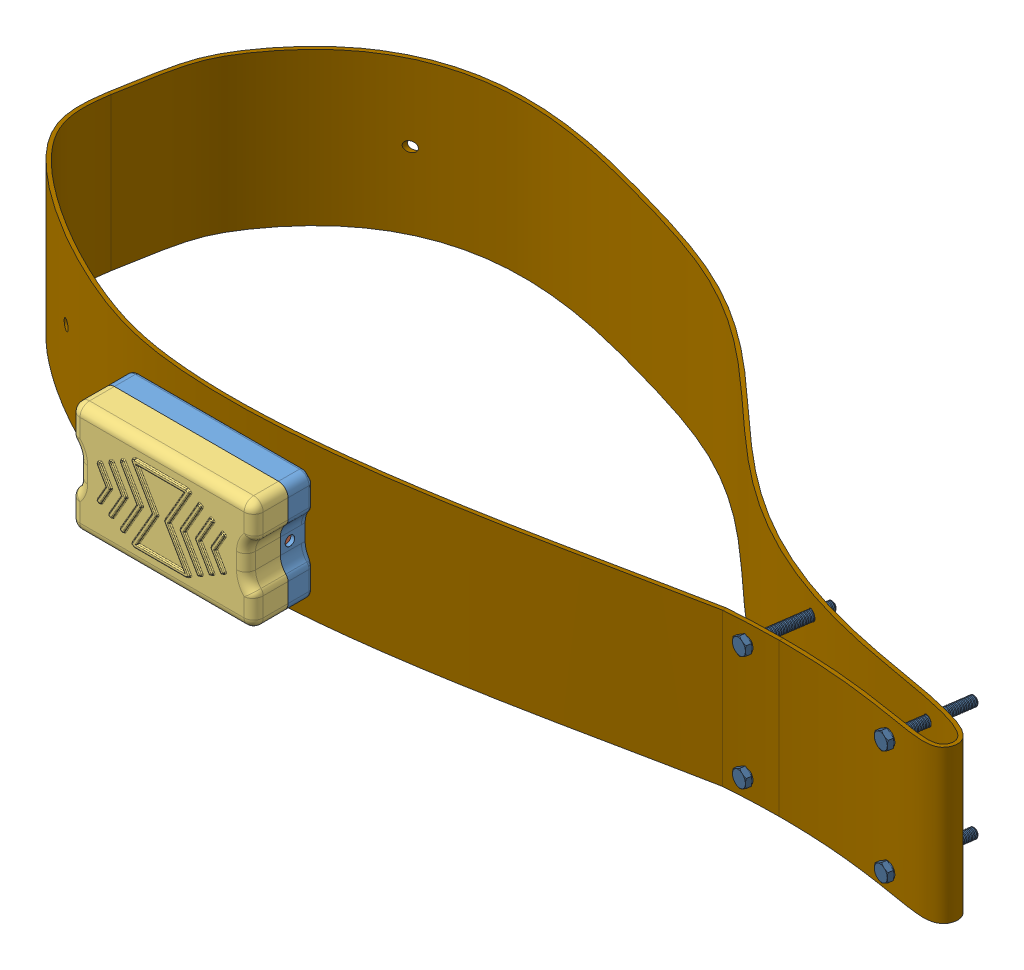
SolidWorks assembly СБ Корпус Peggy Tracker, configuration По умолчанию. Lengths in mm.
Overall size (548.26 80.13 407.1).
306 component instances, 82 part files, 15 mates.
Components (placement in the parent):
- Case-01-1: Case-01 [По умолчанию] at (217.6814 215.7743 273.7334) size (339.05 58 369.63)
- Аккумулятор литий-полимерный LP115181-1: Аккумулятор литий-полимерный LP115181 [Default] at (177.1814 219.2743 275.7334) size (81 51 11)
- Case-02-1: Case-02 [По умолчанию] at (217.6814 215.7743 304.7334) x (-1 0 0) z (0 0 -1) size (96 58 19)
- Печатная плата Peggy Tracker-1: Печатная плата Peggy Tracker [По умолчанию] at (183.6814 227.2743 296.1739) x (0 1 0) z (0 0 -1) size (35 62 10.1)
  - Печатная плата Peggy Tracker.step-1: Печатная плата Peggy Tracker.step [Default] at origin size (35 62 10.1)
    - Board.step-1: Board.step [Default] at origin size (35 62 1.56)
      - Open CASCADE STEP translator 6.8 1.1.1.step-1: Open CASCADE STEP translator 6.8 1.1.1.step [Default] at (0 0 -1.5596) size (35 62 1.56)
    - X1.step-1: X1.step [Default] at origin size (28 20 6.7)
      - 6517451856.step-1: 6517451856.step [Default] at (11.15 51.75 6) size (3 3 0.7)
        - Extruded.step-1: Extruded.step [Default] at origin size (3 3 0.7)
      - 6517450176.step-1: 6517450176.step [Default] at (9.1815 45.8445 6) size (6.22 4.19 0.7)
        - Extruded-0.step-1: Extruded-0.step [Default] at origin size (6.22 4.19 0.7)
      - 6517450176.step-2: 6517450176.step [Default] at (9.1815 57.6545 6) size (6.22 4.19 0.7)
        - Extruded-0.step-1: Extruded-0.step [Default] at origin size (6.22 4.19 0.7)
      - 6517449536.step-1: 6517449536.step [Default] at (4.785 51.7495 0) size (2.57 16 6.7)
        - Extruded-1.step-1: Extruded-1.step [Default] at origin size (2.57 16 6.7)
      - 6517449376.step-1: 6517449376.step [Default] at (8.1819 51.7635 6) size (4.22 2.41 0.7)
        - Extruded-2.step-1: Extruded-2.step [Default] at origin size (4.22 2.41 0.7)
      - 6517449056.step-1: 6517449056.step [Default] at (30.8492 51.7495 0) size (1.3 16 6.7)
        - Extruded-3.step-1: Extruded-3.step [Default] at origin size (1.3 16 6.7)
      - 6517448576.step-1: 6517448576.step [Default] at (28.9305 45.5257 6) size (2.54 3.55 0.7)
        - Extruded-4.step-1: Extruded-4.step [Default] at origin size (2.54 3.55 0.7)
      - 6517448256.step-1: 6517448256.step [Default] at (29.4382 51.4325 6) size (1.52 5.71 0.7)
        - Extruded-5.step-1: Extruded-5.step [Default] at origin size (1.52 5.71 0.7)
      - 6517447856.step-1: 6517447856.step [Default] at (18.1354 51.7495 0) size (24.13 16 1)
        - Extruded-6.step-1: Extruded-6.step [Default] at origin size (24.13 16 1)
      - 6517447456.step-1: 6517447456.step [Default] at (18.135 58.925 0) size (24.13 1.65 2.5)
        - Extruded-7.step-1: Extruded-7.step [Default] at origin size (24.13 1.65 2.5)
      - 6517447456.step-2: 6517447456.step [Default] at (18.1356 44.5737 0) size (24.13 1.65 2.5)
        - Extruded-7.step-1: Extruded-7.step [Default] at origin size (24.13 1.65 2.5)
      - 6517447056.step-1: 6517447056.step [Default] at (19.0875 48.7663 0) size (9.53 0.89 2.5)
        - Extruded-8.step-1: Extruded-8.step [Default] at origin size (9.53 0.89 2.5)
      - 6517447056.step-2: 6517447056.step [Default] at (19.0875 54.2273 0) size (9.53 0.89 2.5)
        - Extruded-8.step-1: Extruded-8.step [Default] at origin size (9.53 0.89 2.5)
      - 6517446256.step-1: 6517446256.step [Default] at (28.9302 57.972 6) size (2.54 3.55 0.7)
        - Extruded-9.step-1: Extruded-9.step [Default] at origin size (2.54 3.55 0.7)
      - CircuitWorks-BATT_CR2032.step-1: CircuitWorks-BATT_CR2032.step [Default] at (17.5 51.75 6) x (1 0 0) z (0 1 0) size (20 3.2 20)
    - XW2.step-1: XW2.step [Default] at origin size (2.86 3.01 1.29)
      - IPX.step-1: IPX.step [Default] at (2.0669 38.1281 1.27) x (0 1 0) z (0 0 1) size (3.01 2.86 1.29)
    - XW1.step-1: XW1.step [Default] at origin size (2.86 3.01 1.29)
      - IPX.step-1: IPX.step [Default] at (1.9653 7.4677 1.27) x (0 1 0) z (0 0 1) size (3.01 2.86 1.29)
    - R6.step-1: R6.step [Default] at origin size (0.9 1.7 0.55)
      - 6482559680.step-1: 6482559680.step [Default] at (28.8001 34.2999 0) x (0 -1 0) z (0 0 1) size (1.7 0.9 0.55)
        - Terminal.step-1: Terminal.step [Default] at (-0.85 -0.45 0) size (0.1 0.9 0.55)
          - Open_CASCADE_STEP_translator_6.8_15.2.1.step-1: Open_CASCADE_STEP_translator_6.8_15.2.1.step [Default] at origin size (0.1 0.9 0.55)
        - Terminal.step-2: Terminal.step [Default] at (0.85 0.45 0) x (-1 0 0) z (0 0 1) size (0.1 0.9 0.55)
          - Open_CASCADE_STEP_translator_6.8_15.2.1.step-1: Open_CASCADE_STEP_translator_6.8_15.2.1.step [Default] at origin size (0.1 0.9 0.55)
        - Mid_Body.step-1: Mid_Body.step [Default] at (-0.85 -0.45 0) size (1.59 0.9 0.44)
        - Mark.step-1: Mark.step [Default] at (-0.75 -0.45 0.495) size (1.5 0.9 0.06)
    - X3.step-1: X3.step [Default] at origin size (4.5 5.9 9.4)
      - B2B-PH-K-S(LF)(SN)--3DModel-STEP-56544.step-1: B2B-PH-K-S(LF)(SN)--3DModel-STEP-56544.step [Default] at (32.5449 33.0001 3) x (0 -1 0) z (-1 0 0) size (5.9 9.4 4.5)
    - R5.step-1: R5.step [Default] at origin size (0.95 1.75 0.95)
      - 6482560720.step-1: 6482560720.step [Default] at (27.1578 23.3326 0) x (0 1 0) z (0 0 1) size (1.75 0.95 0.95)
        - Terminal-1.step-1: Terminal-1.step [Default] at (-0.875 -0.475 0) size (0.2 0.95 0.95)
          - Open_CASCADE_STEP_translator_6.8_12.2.1.step-1: Open_CASCADE_STEP_translator_6.8_12.2.1.step [Default] at origin size (0.2 0.95 0.95)
        - Terminal-1.step-2: Terminal-1.step [Default] at (0.875 0.475 0) x (-1 0 0) z (0 0 1) size (0.2 0.95 0.95)
          - Open_CASCADE_STEP_translator_6.8_12.2.1.step-1: Open_CASCADE_STEP_translator_6.8_12.2.1.step [Default] at origin size (0.2 0.95 0.95)
        - Mid_Body-10.step-1: Mid_Body-10.step [Default] at (-0.875 -0.475 0) size (1.56 0.95 0.76)
        - Mark-11.step-1: Mark-11.step [Default] at (-0.675 -0.475 0.855) size (1.35 0.95 0.1)
    - R4.step-1: R4.step [Default] at origin size (0.95 1.75 0.95)
      - 6482560720.step-1: 6482560720.step [Default] at (27.1578 25.8726 0) x (0 1 0) z (0 0 1) size (1.75 0.95 0.95)
        - Terminal-1.step-1: Terminal-1.step [Default] at (-0.875 -0.475 0) size (0.2 0.95 0.95)
          - Open_CASCADE_STEP_translator_6.8_12.2.1.step-1: Open_CASCADE_STEP_translator_6.8_12.2.1.step [Default] at origin size (0.2 0.95 0.95)
        - Terminal-1.step-2: Terminal-1.step [Default] at (0.875 0.475 0) x (-1 0 0) z (0 0 1) size (0.2 0.95 0.95)
          - Open_CASCADE_STEP_translator_6.8_12.2.1.step-1: Open_CASCADE_STEP_translator_6.8_12.2.1.step [Default] at origin size (0.2 0.95 0.95)
        - Mid_Body-10.step-1: Mid_Body-10.step [Default] at (-0.875 -0.475 0) size (1.56 0.95 0.76)
        - Mark-11.step-1: Mark-11.step [Default] at (-0.675 -0.475 0.855) size (1.35 0.95 0.1)
    - R3.step-1: R3.step [Default] at origin size (0.9 1.7 0.55)
      - 6482559680.step-1: 6482559680.step [Default] at (28.8001 31.7999 0) x (0 -1 0) z (0 0 1) size (1.7 0.9 0.55)
        - Terminal.step-1: Terminal.step [Default] at (-0.85 -0.45 0) size (0.1 0.9 0.55)
          - Open_CASCADE_STEP_translator_6.8_15.2.1.step-1: Open_CASCADE_STEP_translator_6.8_15.2.1.step [Default] at origin size (0.1 0.9 0.55)
        - Terminal.step-2: Terminal.step [Default] at (0.85 0.45 0) x (-1 0 0) z (0 0 1) size (0.1 0.9 0.55)
          - Open_CASCADE_STEP_translator_6.8_15.2.1.step-1: Open_CASCADE_STEP_translator_6.8_15.2.1.step [Default] at origin size (0.1 0.9 0.55)
        - Mid_Body.step-1: Mid_Body.step [Default] at (-0.85 -0.45 0) size (1.59 0.9 0.44)
        - Mark.step-1: Mark.step [Default] at (-0.75 -0.45 0.495) size (1.5 0.9 0.06)
    - R2.step-1: R2.step [Default] at origin size (0.9 1.7 0.55)
      - 6482559840.step-1: 6482559840.step [Default] at (24.5109 16.5497 0) x (0 1 0) z (0 0 1) size (1.7 0.9 0.55)
        - Terminal-2.step-1: Terminal-2.step [Default] at (-0.85 -0.45 0) size (0.1 0.9 0.55)
          - Open_CASCADE_STEP_translator_6.8_15.2.1-12.step-1: Open_CASCADE_STEP_translator_6.8_15.2.1-12.step [Default] at origin size (0.1 0.9 0.55)
        - Terminal-2.step-2: Terminal-2.step [Default] at (0.85 0.45 0) x (-1 0 0) z (0 0 1) size (0.1 0.9 0.55)
          - Open_CASCADE_STEP_translator_6.8_15.2.1-12.step-1: Open_CASCADE_STEP_translator_6.8_15.2.1-12.step [Default] at origin size (0.1 0.9 0.55)
        - Mid_Body-13.step-1: Mid_Body-13.step [Default] at (-0.85 -0.45 0) size (1.59 0.9 0.44)
        - Mark-14.step-1: Mark-14.step [Default] at (-0.75 -0.45 0.495) size (1.5 0.9 0.06)
    - R1.step-1: R1.step [Default] at origin size (1.7 0.9 0.55)
      - 6517452256.step-1: 6517452256.step [Default] at (8.2043 34.8489 0) size (1.7 0.9 0.55)
        - Terminal-3.step-1: Terminal-3.step [Default] at (-0.85 -0.45 0) size (0.1 0.9 0.55)
          - Open_CASCADE_STEP_translator_6.8_15.2.1-15.step-1: Open_CASCADE_STEP_translator_6.8_15.2.1-15.step [Default] at origin size (0.1 0.9 0.55)
        - Terminal-3.step-2: Terminal-3.step [Default] at (0.85 0.45 0) x (-1 0 0) z (0 0 1) size (0.1 0.9 0.55)
          - Open_CASCADE_STEP_translator_6.8_15.2.1-15.step-1: Open_CASCADE_STEP_translator_6.8_15.2.1-15.step [Default] at origin size (0.1 0.9 0.55)
        - Mid_Body-16.step-1: Mid_Body-16.step [Default] at (-0.85 -0.45 0) size (1.59 0.9 0.44)
        - Mark-17.step-1: Mark-17.step [Default] at (-0.75 -0.45 0.495) size (1.5 0.9 0.06)
    - L2.step-1: L2.step [Default] at origin size (5.2 5.2 1.8)
      - 6482573440.step-1: 6482573440.step [Default] at (30.1268 13.8076 0.2) x (1 0 0) z (0 -1 0) size (5.2 1.8 5.2)
    - L1.step-1: L1.step [Default] at origin size (0.95 1.75 0.95)
      - 6482561680.step-1: 6482561680.step [Default] at (5.85 37.366 0) x (0 1 0) z (0 0 1) size (1.75 0.95 0.95)
        - Terminal-4.step-1: Terminal-4.step [Default] at (-0.875 -0.475 0) size (1.75 0.95 0.95)
          - Open_CASCADE_STEP_translator_6.8_2.1.1.step-1: Open_CASCADE_STEP_translator_6.8_2.1.1.step [Default] at origin size (0.2 0.95 0.95)
          - Open_CASCADE_STEP_translator_6.8_2.1.2.step-1: Open_CASCADE_STEP_translator_6.8_2.1.2.step [Default] at origin size (0.2 0.95 0.95)
        - Mid_Body-18.step-1: Mid_Body-18.step [Default] at (-0.875 -0.475 0) size (1.35 0.95 0.95)
          - Open_CASCADE_STEP_translator_6.8_2.2.1.step-1: Open_CASCADE_STEP_translator_6.8_2.2.1.step [Default] at origin size (1.35 0.95 0.95)
    - DD2.step-1: DD2.step [Default] at origin size (15 15.5 3.52)
      - 3D_RAK3172.step-1: 3D_RAK3172.step [Default] at (20.536 20.4601 1) x (-1 0 0) z (0 0 1) size (15 15.5 3.52)
        - Board-1.step-1: Board-1.step [Default] at origin size (15 15.5 1.01)
          - Open_CASCADE_STEP_translator_6.8_1.1.1.step-1: Open_CASCADE_STEP_translator_6.8_1.1.1.step [Default] at (0 0 -1.014) size (15 15.5 1.01)
            - Open_CASCADE_STEP_translator_6.8_1.1.1.1.step-1: Open_CASCADE_STEP_translator_6.8_1.1.1.1.step [Default] at origin size (15 15.5 1.01)
        - R11.step-1: R11.step [Default] at origin size (0.6 0.3 0.3)
          - 0201_SMD_Capacitor.step-1: 0201_SMD_Capacitor.step [Default] at (3.4751 6.9342 0.2794) x (-1 0 0) z (0 0 1) size (0.6 0.3 0.3)
        - U2.step-1: U2.step [Default] at origin size (0.99 1.02 0.75)
          - 6590464912.step-1: 6590464912.step [Default] at (5.4483 13.05 0) size (0.99 1.02 0.75)
            - Extruded-19.step-1: Extruded-19.step [Default] at origin size (0.99 1.02 0.75)
        - R4-1.step-1: R4-1.step [Default] at origin size (0.68 0.33 0.34)
          - R0201.step-1: R0201.step [Default] at (3.9176 5.9192 0) x (1 0 0) z (0 -1 0) size (0.68 0.34 0.33)
        - R3-1.step-1: R3-1.step [Default] at origin size (0.33 0.68 0.34)
          - R0201.step-1: R0201.step [Default] at (4.1676 5.6692 0) x (0 1 0) z (1 0 0) size (0.68 0.34 0.33)
        - L2-1.step-1: L2-1.step [Default] at origin size (1.15 0.55 0.41)
          - RES_1005-0402.step-1: RES_1005-0402.step [Default] at (2.2661 6.0198 0) x (1 0 0) z (0 -1 0) size (1.15 0.41 0.55)
        - C10.step-1: C10.step [Default] at origin size (0.6 0.3 0.3)
          - 0201_SMD_Capacitor.step-1: 0201_SMD_Capacitor.step [Default] at (7.1835 13.462 0.2794) x (-1 0 0) z (0 0 1) size (0.6 0.3 0.3)
        - C9.step-1: C9.step [Default] at origin size (0.6 0.3 0.3)
          - 0201_SMD_Capacitor.step-1: 0201_SMD_Capacitor.step [Default] at (7.1835 13.97 0.2794) x (-1 0 0) z (0 0 1) size (0.6 0.3 0.3)
        - C8.step-1: C8.step [Default] at origin size (0.6 0.3 0.3)
          - 0201_SMD_Capacitor.step-1: 0201_SMD_Capacitor.step [Default] at (7.1835 12.954 0.2794) x (-1 0 0) z (0 0 1) size (0.6 0.3 0.3)
        - C7.step-1: C7.step [Default] at origin size (0.6 0.3 0.3)
          - 0201_SMD_Capacitor.step-1: 0201_SMD_Capacitor.step [Default] at (6.0793 11.938 0.2794) x (1 0 0) z (0 0 1) size (0.6 0.3 0.3)
        - C6.step-1: C6.step [Default] at origin size (0.6 0.3 0.3)
          - 0201_SMD_Capacitor.step-1: 0201_SMD_Capacitor.step [Default] at (3.8855 13.5541 0.2794) x (-1 0 0) z (0 0 1) size (0.6 0.3 0.3)
        - CON1.step-1: CON1.step [Default] at origin size (3.4 3.1 1.25)
          - UFL-R-SMD.step-1: UFL-R-SMD.step [Default] at (11.3537 12.7757 0) x (1 0 0) z (0 0 1) size (3.4 3.1 1.25)
            - Part_525.step-1: Part_525.step [Default] at origin size (3 2.6 0.35)
            - Part_739.step-1: Part_739.step [Default] at origin size (2 2 0.9)
            - Part_578.step-1: Part_578.step [Default] at origin size (0.6 0.5 0.1)
            - Part_540.step-1: Part_540.step [Default] at origin size (0.4 1.8 0.1)
            - Part_562.step-1: Part_562.step [Default] at origin size (0.4 1.8 0.1)
            - Part_555.step-1: Part_555.step [Default] at origin size (0.6 0.5 0.1)
        - C4.step-1: C4.step [Default] at origin size (0.6 0.3 0.3)
          - 0201_SMD_Capacitor.step-1: 0201_SMD_Capacitor.step [Default] at (3.7799 9.398 0.2794) x (-1 0 0) z (0 0 1) size (0.6 0.3 0.3)
        - U1.step-1: U1.step [Default] at origin size (7.02 7.02 0.8)
          - QFN48_7x7.step-1: QFN48_7x7.step [Default] at (8.8366 6.9818 0) x (0 1 0) z (1 0 0) size (7.02 0.8 7.02)
        - X1-1.step-1: X1-1.step [Default] at origin size (1.61 2.01 0.71)
          - NT2016SA.step-1: NT2016SA.step [Default] at (1.7496 8.4946 0) x (0 1 0) z (1 0 0) size (2.01 0.71 1.61)
        - C43.step-1: C43.step [Default] at origin size (0.6 0.3 0.3)
          - 0201_SMD_Capacitor.step-1: 0201_SMD_Capacitor.step [Default] at (3.7799 9.9822 0.2794) x (-1 0 0) z (0 0 1) size (0.6 0.3 0.3)
        - C42.step-1: C42.step [Default] at origin size (0.3 0.6 0.3)
          - 0201_SMD_Capacitor.step-1: 0201_SMD_Capacitor.step [Default] at (3.0734 7.9709 0.2794) x (0 -1 0) z (0 0 1) size (0.6 0.3 0.3)
        - R9.step-1: R9.step [Default] at origin size (0.6 0.3 0.3)
          - 0201_SMD_Capacitor.step-1: 0201_SMD_Capacitor.step [Default] at (3.7799 8.8138 0.2794) x (-1 0 0) z (0 0 1) size (0.6 0.3 0.3)
        - C1.step-1: C1.step [Default] at origin size (0.6 0.3 0.3)
          - 0201_SMD_Capacitor.step-1: 0201_SMD_Capacitor.step [Default] at (7.0445 11.557 0.2794) x (1 0 0) z (0 0 1) size (0.6 0.3 0.3)
        - C2.step-1: C2.step [Default] at origin size (0.3 0.6 0.3)
          - 0201_SMD_Capacitor.step-1: 0201_SMD_Capacitor.step [Default] at (7.9756 12.2635 0.2794) x (0 -1 0) z (0 0 1) size (0.6 0.3 0.3)
        - C3.step-1: C3.step [Default] at origin size (0.3 0.6 0.3)
          - 0201_SMD_Capacitor.step-1: 0201_SMD_Capacitor.step [Default] at (2.1844 13.4518 0.2794) x (0 -1 0) z (0 0 1) size (0.6 0.3 0.3)
        - C11.step-1: C11.step [Default] at origin size (0.6 0.3 0.3)
          - 0201_SMD_Capacitor.step-1: 0201_SMD_Capacitor.step [Default] at (1.6623 11.9866 0.2794) x (1 0 0) z (0 0 1) size (0.6 0.3 0.3)
        - C12.step-1: C12.step [Default] at origin size (0.6 0.3 0.3)
          - 0201_SMD_Capacitor.step-1: 0201_SMD_Capacitor.step [Default] at (3.2813 12.573 0.2794) x (1 0 0) z (0 0 1) size (0.6 0.3 0.3)
        - C13.step-1: C13.step [Default] at origin size (0.3 0.6 0.3)
          - 0201_SMD_Capacitor.step-1: 0201_SMD_Capacitor.step [Default] at (4.4958 12.0697 0.2794) x (0 1 0) z (0 0 1) size (0.6 0.3 0.3)
        - C14.step-1: C14.step [Default] at origin size (0.3 0.6 0.3)
          - 0201_SMD_Capacitor.step-1: 0201_SMD_Capacitor.step [Default] at (2.7178 12.6739 0.2794) x (0 -1 0) z (0 0 1) size (0.6 0.3 0.3)
        - C17.step-1: C17.step [Default] at origin size (0.3 0.6 0.3)
          - 0201_SMD_Capacitor.step-1: 0201_SMD_Capacitor.step [Default] at (7.6708 14.4693 0.2794) x (0 -1 0) z (0 0 1) size (0.6 0.3 0.3)
        - C18.step-1: C18.step [Default] at origin size (0.6 0.3 0.3)
          - 0201_SMD_Capacitor.step-1: 0201_SMD_Capacitor.step [Default] at (9.1901 14.1224 0.2794) x (-1 0 0) z (0 0 1) size (0.6 0.3 0.3)
        - C19.step-1: C19.step [Default] at origin size (0.3 0.6 0.3)
          - 0201_SMD_Capacitor.step-1: 0201_SMD_Capacitor.step [Default] at (2.8814 10.8799 0.2794) x (0 1 0) z (0 0 1) size (0.6 0.3 0.3)
        - C22.step-1: C22.step [Default] at origin size (0.3 0.6 0.3)
          - 0201_SMD_Capacitor.step-1: 0201_SMD_Capacitor.step [Default] at (2.0432 11.4801 0.2794) x (0 -1 0) z (0 0 1) size (0.6 0.3 0.3)
        - C21.step-1: C21.step [Default] at origin size (0.3 0.6 0.3)
          - 0201_SMD_Capacitor.step-1: 0201_SMD_Capacitor.step [Default] at (1.5606 11.4801 0.2794) x (0 -1 0) z (0 0 1) size (0.6 0.3 0.3)
        - C23.step-1: C23.step [Default] at origin size (1 0.5 0.5)
          - C0402.step-1: C0402.step [Default] at (8.9644 1.5539 0.254) x (1 0 0) z (0 0 1) size (1 0.5 0.5)
        - C24.step-1: C24.step [Default] at origin size (0.6 0.3 0.3)
          - 0201_SMD_Capacitor.step-1: 0201_SMD_Capacitor.step [Default] at (4.7197 3.8862 0.2794) x (-1 0 0) z (0 0 1) size (0.6 0.3 0.3)
        - C26.step-1: C26.step [Default] at origin size (0.3 0.6 0.3)
          - 0201_SMD_Capacitor.step-1: 0201_SMD_Capacitor.step [Default] at (10.541 2.2265 0.2794) x (0 -1 0) z (0 0 1) size (0.6 0.3 0.3)
        - C44.step-1: C44.step [Default] at origin size (0.6 0.3 0.3)
          - 0201_SMD_Capacitor.step-1: 0201_SMD_Capacitor.step [Default] at (4.7919 9.9822 0.2794) x (-1 0 0) z (0 0 1) size (0.6 0.3 0.3)
        - C29.step-1: C29.step [Default] at origin size (0.6 0.3 0.3)
          - 0201_SMD_Capacitor.step-1: 0201_SMD_Capacitor.step [Default] at (3.9925 7.8486 0.2794) x (1 0 0) z (0 0 1) size (0.6 0.3 0.3)
        - C25.step-1: C25.step [Default] at origin size (0.3 0.6 0.3)
          - 0201_SMD_Capacitor.step-1: 0201_SMD_Capacitor.step [Default] at (10.287 1.6263 0.2794) x (0 1 0) z (0 0 1) size (0.6 0.3 0.3)
        - C31.step-1: C31.step [Default] at origin size (0.6 0.3 0.3)
          - 0201_SMD_Capacitor.step-1: 0201_SMD_Capacitor.step [Default] at (3.9965 7.239 0.2794) x (1 0 0) z (0 0 1) size (0.6 0.3 0.3)
        - C32.step-1: C32.step [Default] at origin size (0.6 0.3 0.3)
          - 0201_SMD_Capacitor.step-1: 0201_SMD_Capacitor.step [Default] at (7.8533 2.3622 0.2794) x (1 0 0) z (0 0 1) size (0.6 0.3 0.3)
        - C33.step-1: C33.step [Default] at origin size (1 0.5 0.5)
          - C0402.step-1: C0402.step [Default] at (5.3048 2.0461 0.254) x (-1 0 0) z (0 0 1) size (1 0.5 0.5)
        - C34.step-1: C34.step [Default] at origin size (0.3 0.6 0.3)
          - 0201_SMD_Capacitor.step-1: 0201_SMD_Capacitor.step [Default] at (4.318 4.2211 0.2794) x (0 1 0) z (0 0 1) size (0.6 0.3 0.3)
        - C35.step-1: C35.step [Default] at origin size (0.6 0.3 0.3)
          - 0201_SMD_Capacitor.step-1: 0201_SMD_Capacitor.step [Default] at (9.0365 2.3622 0.2794) x (1 0 0) z (0 0 1) size (0.6 0.3 0.3)
        - C36.step-1: C36.step [Default] at origin size (0.3 0.6 0.3)
          - 0201_SMD_Capacitor.step-1: 0201_SMD_Capacitor.step [Default] at (13.0302 10.0751 0.2794) x (0 -1 0) z (0 0 1) size (0.6 0.3 0.3)
        - C37.step-1: C37.step [Default] at origin size (0.3 0.6 0.3)
          - 0201_SMD_Capacitor.step-1: 0201_SMD_Capacitor.step [Default] at (3.7338 4.2211 0.2794) x (0 1 0) z (0 0 1) size (0.6 0.3 0.3)
        - C38.step-1: C38.step [Default] at origin size (1 0.5 0.5)
          - C0402.step-1: C0402.step [Default] at (2.3114 4.7323 0.254) x (1 0 0) z (0 0 1) size (1 0.5 0.5)
        - C39.step-1: C39.step [Default] at origin size (0.6 0.3 0.3)
          - 0201_SMD_Capacitor.step-1: 0201_SMD_Capacitor.step [Default] at (4.0593 3.1881 0.2794) x (-1 0 0) z (0 0 1) size (0.6 0.3 0.3)
        - C40.step-1: C40.step [Default] at origin size (0.3 0.6 0.3)
          - 0201_SMD_Capacitor.step-1: 0201_SMD_Capacitor.step [Default] at (3.6576 1.7319 0.2794) x (0 1 0) z (0 0 1) size (0.6 0.3 0.3)
        - L1-1.step-1: L1-1.step [Default] at origin size (0.68 0.33 0.34)
          - R0201.step-1: R0201.step [Default] at (7.8526 11.2014 0) x (-1 0 0) z (0 1 0) size (0.68 0.34 0.33)
        - L3.step-1: L3.step [Default] at origin size (0.33 0.68 0.34)
          - R0201.step-1: R0201.step [Default] at (1.7272 13.1318 0) x (0 -1 0) z (-1 0 0) size (0.68 0.34 0.33)
        - L5.step-1: L5.step [Default] at origin size (0.68 0.33 0.34)
          - R0201.step-1: R0201.step [Default] at (8.0772 13.3096 0) x (-1 0 0) z (0 1 0) size (0.68 0.34 0.33)
        - L6.step-1: L6.step [Default] at origin size (1 0.5 0.5)
          - C0402.step-1: C0402.step [Default] at (5.822 11.0823 0.254) x (1 0 0) z (0 0 1) size (1 0.5 0.5)
        - L7.step-1: L7.step [Default] at origin size (0.68 0.33 0.34)
          - R0201.step-1: R0201.step [Default] at (3.5854 12.1158 0) x (1 0 0) z (0 -1 0) size (0.68 0.34 0.33)
        - L9.step-1: L9.step [Default] at origin size (1.15 0.55 0.41)
          - RES_1005-0402.step-1: RES_1005-0402.step [Default] at (3.9641 11.3538 0) x (-1 0 0) z (0 1 0) size (1.15 0.41 0.55)
        - L20.step-1: L20.step [Default] at origin size (1.6 0.8 0.3)
          - 6559637360.step-1: 6559637360.step [Default] at (12.3698 2.0828 0) x (-1 0 0) z (0 1 0) size (1.6 0.3 0.8)
        - L30.step-1: L30.step [Default] at origin size (1.15 0.55 0.41)
          - RES_1005-0402.step-1: RES_1005-0402.step [Default] at (7.1263 1.8 0) x (-1 0 0) z (0 1 0) size (1.15 0.41 0.55)
        - X2.step-1: X2.step [Default] at origin size (1.2 2 0.61)
          - crystal_rtf2012.step-1: crystal_rtf2012.step [Default] at (2.25 2.8402 0) x (0 1 0) z (1 0 0) size (2 0.61 1.2)
        - R2-1.step-1: R2-1.step [Default] at origin size (0.68 0.33 0.34)
          - R0201.step-1: R0201.step [Default] at (1.9613 10.1854 0) x (1 0 0) z (0 -1 0) size (0.68 0.34 0.33)
        - C5.step-1: C5.step [Default] at origin size (0.6 0.3 0.3)
          - 0201_SMD_Capacitor.step-1: 0201_SMD_Capacitor.step [Default] at (1.8749 6.9342 0.2794) x (-1 0 0) z (0 0 1) size (0.6 0.3 0.3)
        - Free-Models.step-1: Free-Models.step [Default] at origin size (13.4 13.9 2.5)
          - D030A-______.step-1: D030A-______.step [Default] at (2.429 -1.8288 0) size (13.4 13.9 2.5)
    - DD1.step-1: DD1.step [Default] at origin size (9.7 10.1 2.8)
      - 6482566000.step-1: 6482566000.step [Default] at (16.1 34.85 0) x (1 0 0) z (0 0 1) size (9.7 10.1 2.8)
        - Body.step-1: Body.step [Default] at (0 0 0.1) size (9.7 10.1 2.7)
        - Pins.step-1: Pins.step [Default] at origin size (9.56 9.36 0.1)
    - DA1.step-1: DA1.step [Default] at origin size (3 3 1)
      - 6482561360.step-1: 6482561360.step [Default] at (31.2728 20.6686 0) x (0 1 0) z (0 0 1) size (3 3 1)
        - FRAME-DRC0010J.step-1: FRAME-DRC0010J.step [Default] x (1 0 0) z (0 -1 0) size (3 0.2 3)
          - Open CASCADE STEP translator 6.8 1.16.1.2.1.step-1: Open CASCADE STEP translator 6.8 1.16.1.2.1.step [Default] at origin size (1.9 0.2 3)
          - Open CASCADE STEP translator 6.8 1.16.1.2.2.step-1: Open CASCADE STEP translator 6.8 1.16.1.2.2.step [Default] at origin size (0.4 0.2 0.24)
          - Open CASCADE STEP translator 6.8 1.16.1.2.3.step-1: Open CASCADE STEP translator 6.8 1.16.1.2.3.step [Default] at origin size (0.4 0.2 0.24)
          - Open CASCADE STEP translator 6.8 1.16.1.2.4.step-1: Open CASCADE STEP translator 6.8 1.16.1.2.4.step [Default] at origin size (0.4 0.2 0.24)
          - Open CASCADE STEP translator 6.8 1.16.1.2.5.step-1: Open CASCADE STEP translator 6.8 1.16.1.2.5.step [Default] at origin size (0.4 0.2 0.24)
          - Open CASCADE STEP translator 6.8 1.16.1.2.6.step-1: Open CASCADE STEP translator 6.8 1.16.1.2.6.step [Default] at origin size (0.4 0.2 0.24)
          - Open CASCADE STEP translator 6.8 1.16.1.2.7.step-1: Open CASCADE STEP translator 6.8 1.16.1.2.7.step [Default] at origin size (0.4 0.2 0.24)
          - Open CASCADE STEP translator 6.8 1.16.1.2.8.step-1: Open CASCADE STEP translator 6.8 1.16.1.2.8.step [Default] at origin size (0.4 0.2 0.24)
          - Open CASCADE STEP translator 6.8 1.16.1.2.9.step-1: Open CASCADE STEP translator 6.8 1.16.1.2.9.step [Default] at origin size (0.4 0.2 0.24)
          - Open CASCADE STEP translator 6.8 1.16.1.2.10.step-1: Open CASCADE STEP translator 6.8 1.16.1.2.10.step [Default] at origin size (0.4 0.2 0.24)
          - Open CASCADE STEP translator 6.8 1.16.1.2.11.step-1: Open CASCADE STEP translator 6.8 1.16.1.2.11.step [Default] at origin size (0.4 0.2 0.24)
        - BODY-SON.step-1: BODY-SON.step [Default] at (0 0 0.025) x (1 0 0) z (0 -1 0) size (3 0.97 3)
    - C8-1.step-1: C8-1.step [Default] at origin size (1.4 2.15 1.4)
      - 6482573680.step-1: 6482573680.step [Default] at (27.1929 19.9035 0) x (0 -1 0) z (0 0 1) size (2.15 1.4 1.4)
        - Terminal-5.step-1: Terminal-5.step [Default] at (-1.075 -0.7 0) size (2.15 1.4 1.4)
          - Open_CASCADE_STEP_translator_6.8_5.1.1.step-1: Open_CASCADE_STEP_translator_6.8_5.1.1.step [Default] at origin size (0.2 1.4 1.4)
          - Open_CASCADE_STEP_translator_6.8_5.1.2.step-1: Open_CASCADE_STEP_translator_6.8_5.1.2.step [Default] at origin size (0.2 1.4 1.4)
        - Mid_Body-1.step-1: Mid_Body-1.step [Default] at (-1.075 -0.7 0) size (1.75 1.4 1.4)
          - Open_CASCADE_STEP_translator_6.8_5.2.1.step-1: Open_CASCADE_STEP_translator_6.8_5.2.1.step [Default] at origin size (1.75 1.4 1.4)
    - C7-1.step-1: C7-1.step [Default] at origin size (2.1 1.35 1.35)
      - 6482573600.step-1: 6482573600.step [Default] at (31.889 26.8 0) x (1 0 0) z (0 0 1) size (2.1 1.35 1.35)
        - Terminal-6.step-1: Terminal-6.step [Default] at (-1.05 -0.675 0) size (2.1 1.35 1.35)
          - Open_CASCADE_STEP_translator_6.8_24.1.1.step-1: Open_CASCADE_STEP_translator_6.8_24.1.1.step [Default] at origin size (0.2 1.35 1.35)
          - Open_CASCADE_STEP_translator_6.8_24.1.2.step-1: Open_CASCADE_STEP_translator_6.8_24.1.2.step [Default] at origin size (0.2 1.35 1.35)
        - Mid_Body-2.step-1: Mid_Body-2.step [Default] at (-1.05 -0.675 0) size (1.7 1.35 1.35)
          - Open_CASCADE_STEP_translator_6.8_24.2.1.step-1: Open_CASCADE_STEP_translator_6.8_24.2.1.step [Default] at origin size (1.7 1.35 1.35)
    - C6-1.step-1: C6-1.step [Default] at origin size (0.9 1.7 0.9)
      - 6482559520.step-1: 6482559520.step [Default] at (22.727 16.763 0) x (0 -1 0) z (0 0 1) size (1.7 0.9 0.9)
        - Terminal-7.step-1: Terminal-7.step [Default] at (-0.85 -0.45 0) size (1.7 0.9 0.9)
          - Open_CASCADE_STEP_translator_6.8_5.1.1-20.step-1: Open_CASCADE_STEP_translator_6.8_5.1.1-20.step [Default] at origin size (0.2 0.9 0.9)
          - Open_CASCADE_STEP_translator_6.8_5.1.2-21.step-1: Open_CASCADE_STEP_translator_6.8_5.1.2-21.step [Default] at origin size (0.2 0.9 0.9)
        - Mid_Body-3.step-1: Mid_Body-3.step [Default] at (-0.85 -0.45 0) size (1.3 0.9 0.9)
          - Open_CASCADE_STEP_translator_6.8_5.2.1-22.step-1: Open_CASCADE_STEP_translator_6.8_5.2.1-22.step [Default] at origin size (1.3 0.9 0.9)
    - C5-1.step-1: C5-1.step [Default] at origin size (1.35 2.1 1.35)
      - 6482568960.step-1: 6482568960.step [Default] at (24.505 19.939 0) x (0 -1 0) z (0 0 1) size (2.1 1.35 1.35)
        - Terminal-8.step-1: Terminal-8.step [Default] at (-1.05 -0.675 0) size (2.1 1.35 1.35)
          - Open_CASCADE_STEP_translator_6.8_24.1.1-23.step-1: Open_CASCADE_STEP_translator_6.8_24.1.1-23.step [Default] at origin size (0.2 1.35 1.35)
          - Open_CASCADE_STEP_translator_6.8_24.1.2-24.step-1: Open_CASCADE_STEP_translator_6.8_24.1.2-24.step [Default] at origin size (0.2 1.35 1.35)
        - Mid_Body-4.step-1: Mid_Body-4.step [Default] at (-1.05 -0.675 0) size (1.7 1.35 1.35)
          - Open_CASCADE_STEP_translator_6.8_24.2.1-25.step-1: Open_CASCADE_STEP_translator_6.8_24.2.1-25.step [Default] at origin size (1.7 1.35 1.35)
    - C4-1.step-1: C4-1.step [Default] at origin size (0.9 1.7 0.9)
      - 6482559520.step-1: 6482559520.step [Default] at (22.7 19.888 0) x (0 -1 0) z (0 0 1) size (1.7 0.9 0.9)
        - Terminal-7.step-1: Terminal-7.step [Default] at (-0.85 -0.45 0) size (1.7 0.9 0.9)
          - Open_CASCADE_STEP_translator_6.8_5.1.1-20.step-1: Open_CASCADE_STEP_translator_6.8_5.1.1-20.step [Default] at origin size (0.2 0.9 0.9)
          - Open_CASCADE_STEP_translator_6.8_5.1.2-21.step-1: Open_CASCADE_STEP_translator_6.8_5.1.2-21.step [Default] at origin size (0.2 0.9 0.9)
        - Mid_Body-3.step-1: Mid_Body-3.step [Default] at (-0.85 -0.45 0) size (1.3 0.9 0.9)
          - Open_CASCADE_STEP_translator_6.8_5.2.1-22.step-1: Open_CASCADE_STEP_translator_6.8_5.2.1-22.step [Default] at origin size (1.3 0.9 0.9)
    - C3-1.step-1: C3-1.step [Default] at origin size (1.35 2.1 1.35)
      - 6482568960.step-1: 6482568960.step [Default] at (25.7048 39.0008 0) x (0 -1 0) z (0 0 1) size (2.1 1.35 1.35)
        - Terminal-8.step-1: Terminal-8.step [Default] at (-1.05 -0.675 0) size (2.1 1.35 1.35)
          - Open_CASCADE_STEP_translator_6.8_24.1.1-23.step-1: Open_CASCADE_STEP_translator_6.8_24.1.1-23.step [Default] at origin size (0.2 1.35 1.35)
          - Open_CASCADE_STEP_translator_6.8_24.1.2-24.step-1: Open_CASCADE_STEP_translator_6.8_24.1.2-24.step [Default] at origin size (0.2 1.35 1.35)
        - Mid_Body-4.step-1: Mid_Body-4.step [Default] at (-1.05 -0.675 0) size (1.7 1.35 1.35)
          - Open_CASCADE_STEP_translator_6.8_24.2.1-25.step-1: Open_CASCADE_STEP_translator_6.8_24.2.1-25.step [Default] at origin size (1.7 1.35 1.35)
    - C2-1.step-1: C2-1.step [Default] at origin size (0.9 1.7 0.9)
      - 6482561200.step-1: 6482561200.step [Default] at (23.5204 39.0508 0) x (0 1 0) z (0 0 1) size (1.7 0.9 0.9)
        - Terminal-9.step-1: Terminal-9.step [Default] at (-0.85 -0.45 0) size (1.7 0.9 0.9)
          - Open_CASCADE_STEP_translator_6.8_5.1.1-26.step-1: Open_CASCADE_STEP_translator_6.8_5.1.1-26.step [Default] at origin size (0.2 0.9 0.9)
          - Open_CASCADE_STEP_translator_6.8_5.1.2-27.step-1: Open_CASCADE_STEP_translator_6.8_5.1.2-27.step [Default] at origin size (0.2 0.9 0.9)
        - Mid_Body-5.step-1: Mid_Body-5.step [Default] at (-0.85 -0.45 0) size (1.3 0.9 0.9)
          - Open_CASCADE_STEP_translator_6.8_5.2.1-28.step-1: Open_CASCADE_STEP_translator_6.8_5.2.1-28.step [Default] at origin size (1.3 0.9 0.9)
    - C1-1.step-1: C1-1.step [Default] at origin size (0.9 1.7 0.9)
      - 6482559520.step-1: 6482559520.step [Default] at (5.842 33.9488 0) x (0 -1 0) z (0 0 1) size (1.7 0.9 0.9)
        - Terminal-7.step-1: Terminal-7.step [Default] at (-0.85 -0.45 0) size (1.7 0.9 0.9)
          - Open_CASCADE_STEP_translator_6.8_5.1.1-20.step-1: Open_CASCADE_STEP_translator_6.8_5.1.1-20.step [Default] at origin size (0.2 0.9 0.9)
          - Open_CASCADE_STEP_translator_6.8_5.1.2-21.step-1: Open_CASCADE_STEP_translator_6.8_5.1.2-21.step [Default] at origin size (0.2 0.9 0.9)
        - Mid_Body-3.step-1: Mid_Body-3.step [Default] at (-0.85 -0.45 0) size (1.3 0.9 0.9)
          - Open_CASCADE_STEP_translator_6.8_5.2.1-22.step-1: Open_CASCADE_STEP_translator_6.8_5.2.1-22.step [Default] at origin size (1.3 0.9 0.9)
- Ремень-1: Ремень [По умолчанию] at (467.2058 244.7743 293.1371) x (0.989893 0 0.141813) z (0 1 0) size (523.86 209.36 80.13)
- Hexagon Head Bolt DIN М5-1: Hexagon Head Bolt DIN М5 [DIN 933 - M8X45mm] at (457.3093 274.7743 242.0844) x (0.141813 0 -0.989893) z (-0.51401 0.854618 -0.073638) size (43.5 9.24 8)
- Hexagon Head Bolt DIN М5-2: Hexagon Head Bolt DIN М5 [DIN 933 - M8X45mm] at (457.3093 214.7743 242.0844) x (0.141813 0 -0.989893) z (0.51401 0.854618 0.073638) size (43.5 9.24 8)
- Hexagon Head Bolt DIN М5-3: Hexagon Head Bolt DIN М5 [DIN 933 - M8X45mm] at (537.3151 274.7743 247.7454) x (0.141813 0 -0.989893) z (0.989893 0 0.141813) size (43.5 9.24 8)
- Hexagon Head Bolt DIN М5-4: Hexagon Head Bolt DIN М5 [DIN 933 - M8X45mm] at (537.3151 214.7743 247.7454) x (0.141813 0 -0.989893) z (-0.989893 0 -0.141813) size (43.5 9.24 8)
Mates (geometry in assembly coordinates):
- Coincident1: coincident anti-aligned: plane of Case-01-1 through (217.6814 215.7743 275.7334) normal (0 0 1); plane of Аккумулятор литий-полимерный LP115181-1 through (177.1814 219.2743 275.7334) normal (0 0 -1)
- Width1: width anti-aligned: plane of Case-01-1 through (259.6814 234.7743 286.7334) normal (-1 0 0); plane of Аккумулятор литий-полимерный LP115181-1 through (175.6814 234.7743 286.7334) normal (1 0 0); plane of Case-01-1 through (258.1814 219.2743 286.7334) normal (1 0 0); plane of Аккумулятор литий-полимерный LP115181-1 through (177.1814 219.2743 286.7334) normal (-1 0 0)
- Width2: width anti-aligned: plane of Case-01-1 through (169.6814 271.7743 286.7334) normal (0 -1 0); plane of Аккумулятор литий-полимерный LP115181-1 through (265.6814 217.7743 286.7334) normal (0 1 0); plane of Case-01-1 through (177.1814 270.2743 286.7334) normal (0 1 0); plane of Аккумулятор литий-полимерный LP115181-1 through (177.1814 219.2743 286.7334) normal (0 -1 0)
- Concentric1: concentric aligned: cylinder of Case-02-1 through (246.6814 260.2743 297.7334) axis (0 0 1) radius 1.25; cylinder of Печатная плата Peggy Tracker-1/Печатная плата Peggy Tracker.step-1/Board.step-1/Open CASCADE STEP translator 6.8 1.1.1.step-1 through (246.6814 260.2743 297.7334) axis (0 0 1) radius 1.25
- Concentric2: concentric aligned: cylinder of Case-02-1 through (188.6814 260.2743 297.7334) axis (0 0 1) radius 1.25; cylinder of Печатная плата Peggy Tracker-1/Печатная плата Peggy Tracker.step-1/Board.step-1/Open CASCADE STEP translator 6.8 1.1.1.step-1 through (188.6814 260.2743 297.7334) axis (0 0 1) radius 1.25
- Coincident2: coincident anti-aligned: plane of Case-02-1 through (188.6814 260.2743 297.7334) normal (0 0 -1); plane of Печатная плата Peggy Tracker-1/Печатная плата Peggy Tracker.step-1/Board.step-1/Open CASCADE STEP translator 6.8 1.1.1.step-1 through (186.6814 227.2743 297.7334) normal (0 0 1)
- Coincident6: coincident anti-aligned: plane of Case-01-1 through (217.6814 215.7743 286.7334) normal (0 0 1); plane of Case-02-1 through (217.6814 215.7743 286.7334) normal (0 0 -1)
- Coincident4: coincident aligned: plane of Case-01-1 through (169.6814 254.7743 286.7334) normal (-1 0 0); plane of Case-02-1 through (169.6814 254.7743 286.7334) normal (-1 0 0)
- Coincident5: coincident aligned: plane of Case-01-1 through (169.6814 273.7743 286.7334) normal (0 1 0); plane of Case-02-1 through (265.6814 273.7743 286.7334) normal (0 1 0)
- Tangent5: tangent anti-aligned: plane of Case-01-1 through (217.6814 215.7743 273.7334) normal (0 0 -1); face of Ремень-1
- Width4: width aligned: plane of Case-01-1 through (169.6814 273.7743 286.7334) normal (0 1 0); plane of Ремень-1 through (265.6814 215.7743 286.7334) normal (0 -1 0); plane of Case-01-1 through (446.7006 284.7743 239.8564) normal (0 1 0); plane of Ремень-1 through (446.7006 204.7743 239.8564) normal (0 -1 0)
- Concentric4: concentric aligned: cylinder of Ремень-1 through (467.3592 274.7743 171.9339) axis (-0.141813 0 0.989893) radius 2.65; cylinder of Hexagon Head Bolt DIN М5-1 through (457.3093 274.7743 242.0844) axis (-0.141813 0 0.989893) radius 2.5
- Tangent7: tangent: circle of assembly; face of Ремень-1; circle of Hexagon Head Bolt DIN М5-1
- Concentric5: concentric aligned: cylinder of Ремень-1 through (546.5506 274.7743 183.279) axis (-0.141813 0 0.989893) radius 2.65; cone of Hexagon Head Bolt DIN М5-3 through (538.2156 274.7743 241.4594) axis (-0.141813 0 0.989893)
- Tangent8: tangent: plane of assembly; face of Ремень-1; plane of Hexagon Head Bolt DIN М5-3 through (537.8115 279.3931 244.2807) normal (0.141813 0 -0.989893)
